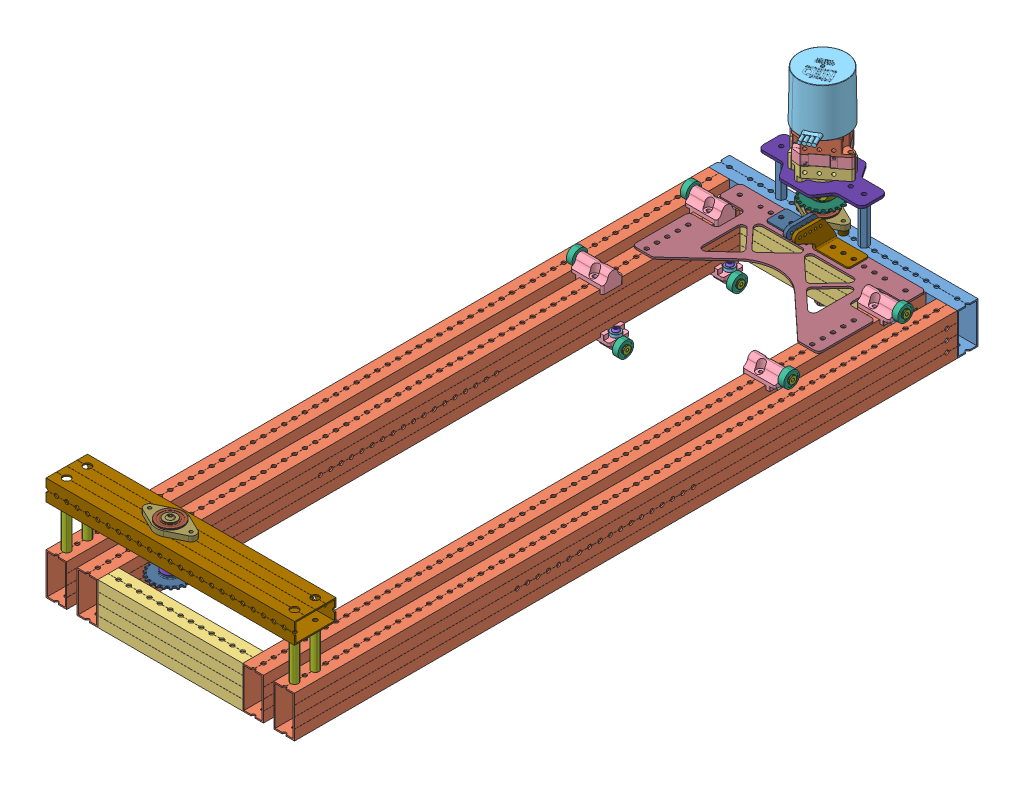
SolidWorks assembly Elevator Assembly Updated 2.0, configuration Default. Lengths in mm.
Overall size (304.8 250.34 871.89).
92 component instances, 31 part files, 131 mates.
Components (placement in the parent):
- WCP-EX-0018-001(2)^Assem1-1: WCP-EX-0018-001(2)^Assem1 [Default] at (184.7308 227.7739 250.3499) size (304.8 50.8 25.4)
- WCP-EX-0018-005(2)^Assem1-1: WCP-EX-0018-005(2)^Assem1 [Default] at (45.0308 227.7739 859.9499) x (0 0 -1) z (1 0 0) size (812.8 50.8 25.4)
- WCP-EX-0018-004(2)^Assem1-1: WCP-EX-0018-004(2)^Assem1 [Default] at (184.7308 227.7739 1063.1499) size (177.8 50.8 25.4)
- WCP-EX-0018-005(2)^Assem1-2: WCP-EX-0018-005(2)^Assem1 [Default] at (324.4308 227.7739 859.9499) x (0 0 -1) z (1 0 0) size (812.8 50.8 25.4)
- WCP-EX-0018-005(2)^Assem1-3: WCP-EX-0018-005(2)^Assem1 [Default] at (286.3308 227.7739 859.9499) x (0 0 -1) z (1 0 0) size (812.8 50.8 25.4)
- WCP-EX-0018-005(2)^Assem1-4: WCP-EX-0018-005(2)^Assem1 [Default] at (83.1308 227.7739 859.9499) x (0 0 -1) z (1 0 0) size (812.8 50.8 25.4)
- WCP-EX-0018-004(2)^Assem1-2: WCP-EX-0018-004(2)^Assem1 [Default] at (184.7308 227.7739 275.7499) size (177.8 50.8 25.4)
- Copy of WCP-0323 - Elevator Clamping Block-1-1: Copy of WCP-0323 - Elevator Clamping Block-1 [Default] at (70.4308 253.1739 307.4999) x (0 -1 0) z (-1 0 0) size (29.22 25.41 49.35)
  - WCP-0323-001 Rev2^Copy of WCP-0323 - Elevator Clamping Block-1-1: WCP-0323-001 Rev2^Copy of WCP-0323 - Elevator Clamping Block-1 [Default] at origin size (20.38 25.41 40.49) (virtual)
  - WCP-0498 Rev1^Copy of WCP-0323 - Elevator Clamping Block-1-1: WCP-0498 Rev1^Copy of WCP-0323 - Elevator Clamping Block-1 [Default] at (2.254 0 6.7) x (0 0.307359 0.951594) z (-1 0 0) size (12 12 4) (virtual)
  - WCP-0212_0_250_radial_bearing^Copy of WCP-0323 - Elevator Clamping Block-1-1: WCP-0212_0_250_radial_bearing^Copy of WCP-0323 - Elevator Clamping Block-1 [Default] at (-9.525 0 15.4781) size (19.05 19.05 7.14) (virtual)
  - WCP-0473 Rev1^Copy of WCP-0323 - Elevator Clamping Block-1-1: WCP-0473 Rev1^Copy of WCP-0323 - Elevator Clamping Block-1 [Default] at (-9.525 0 10.4394) x (-0.082744 -0.996571 0) z (-0.996571 0.082744 0) size (9.53 20.65 9.53) (virtual)
  - #8-32 x .25L BHCS^Copy of WCP-0323 - Elevator Clamping Block-1-1: #8-32 x .25L BHCS^Copy of WCP-0323 - Elevator Clamping Block-1 [Default] at (6.7178 0 6.7) x (0 -0.337236 -0.94142) z (1 0 0) size (10.28 8 12.02) (virtual)
- WCP-0583-025 Rev1_DefaultSM-FLAT-PATTERN(2)^Elevator Assembly Updated 2.0-1: WCP-0583-025 Rev1_DefaultSM-FLAT-PATTERN(2)^Elevator Assembly Updated 2.0 [Default] at (206.9558 257.1739 275.7499) x (-1 0 0) z (0 1 0) size (44.45 50.8 31.75) (virtual)
- WCP-0583-026 Rev1(2)^Elevator Assembly Updated 2.0-1: WCP-0583-026 Rev1(2)^Elevator Assembly Updated 2.0 [Default] at (152.9808 257.1739 275.7499) x (-1 0 0) z (0 1 0) size (50.8 50.8 31.75) (virtual)
- Copy of WCP-0323 - Elevator Clamping Block-1-2: Copy of WCP-0323 - Elevator Clamping Block-1 [Default] at (70.4308 253.1739 447.1999) x (0 -1 0) z (-1 0 0) size (29.22 25.41 49.35)
  - WCP-0323-001 Rev2^Copy of WCP-0323 - Elevator Clamping Block-1-1: WCP-0323-001 Rev2^Copy of WCP-0323 - Elevator Clamping Block-1 [Default] at origin size (20.38 25.41 40.49) (virtual)
  - WCP-0498 Rev1^Copy of WCP-0323 - Elevator Clamping Block-1-1: WCP-0498 Rev1^Copy of WCP-0323 - Elevator Clamping Block-1 [Default] at (2.254 0 6.7) x (0 0.307359 0.951594) z (-1 0 0) size (12 12 4) (virtual)
  - WCP-0212_0_250_radial_bearing^Copy of WCP-0323 - Elevator Clamping Block-1-1: WCP-0212_0_250_radial_bearing^Copy of WCP-0323 - Elevator Clamping Block-1 [Default] at (-9.525 0 15.4781) size (19.05 19.05 7.14) (virtual)
  - WCP-0473 Rev1^Copy of WCP-0323 - Elevator Clamping Block-1-1: WCP-0473 Rev1^Copy of WCP-0323 - Elevator Clamping Block-1 [Default] at (-9.525 0 10.4394) x (-0.082744 -0.996571 0) z (-0.996571 0.082744 0) size (9.53 20.65 9.53) (virtual)
  - #8-32 x .25L BHCS^Copy of WCP-0323 - Elevator Clamping Block-1-1: #8-32 x .25L BHCS^Copy of WCP-0323 - Elevator Clamping Block-1 [Default] at (6.7178 0 6.7) x (0 -0.337236 -0.94142) z (1 0 0) size (10.28 8 12.02) (virtual)
- Copy of WCP-0323 - Elevator Clamping Block-1-3: Copy of WCP-0323 - Elevator Clamping Block-1 [Default] at (299.0308 253.1739 447.1999) x (0 -1 0) z (1 0 0) size (29.22 25.41 49.35)
  - WCP-0323-001 Rev2^Copy of WCP-0323 - Elevator Clamping Block-1-1: WCP-0323-001 Rev2^Copy of WCP-0323 - Elevator Clamping Block-1 [Default] at origin size (20.38 25.41 40.49) (virtual)
  - WCP-0498 Rev1^Copy of WCP-0323 - Elevator Clamping Block-1-1: WCP-0498 Rev1^Copy of WCP-0323 - Elevator Clamping Block-1 [Default] at (2.254 0 6.7) x (0 0.307359 0.951594) z (-1 0 0) size (12 12 4) (virtual)
  - WCP-0212_0_250_radial_bearing^Copy of WCP-0323 - Elevator Clamping Block-1-1: WCP-0212_0_250_radial_bearing^Copy of WCP-0323 - Elevator Clamping Block-1 [Default] at (-9.525 0 15.4781) size (19.05 19.05 7.14) (virtual)
  - WCP-0473 Rev1^Copy of WCP-0323 - Elevator Clamping Block-1-1: WCP-0473 Rev1^Copy of WCP-0323 - Elevator Clamping Block-1 [Default] at (-9.525 0 10.4394) x (-0.082744 -0.996571 0) z (-0.996571 0.082744 0) size (9.53 20.65 9.53) (virtual)
  - #8-32 x .25L BHCS^Copy of WCP-0323 - Elevator Clamping Block-1-1: #8-32 x .25L BHCS^Copy of WCP-0323 - Elevator Clamping Block-1 [Default] at (6.7178 0 6.7) x (0 -0.337236 -0.94142) z (1 0 0) size (10.28 8 12.02) (virtual)
- Copy of WCP-0323 - Elevator Clamping Block-1-4: Copy of WCP-0323 - Elevator Clamping Block-1 [Default] at (299.0308 253.1739 307.4999) x (0 -1 0) z (1 0 0) size (29.22 25.41 49.35)
  - WCP-0323-001 Rev2^Copy of WCP-0323 - Elevator Clamping Block-1-1: WCP-0323-001 Rev2^Copy of WCP-0323 - Elevator Clamping Block-1 [Default] at origin size (20.38 25.41 40.49) (virtual)
  - WCP-0498 Rev1^Copy of WCP-0323 - Elevator Clamping Block-1-1: WCP-0498 Rev1^Copy of WCP-0323 - Elevator Clamping Block-1 [Default] at (2.254 0 6.7) x (0 0.307359 0.951594) z (-1 0 0) size (12 12 4) (virtual)
  - WCP-0212_0_250_radial_bearing^Copy of WCP-0323 - Elevator Clamping Block-1-1: WCP-0212_0_250_radial_bearing^Copy of WCP-0323 - Elevator Clamping Block-1 [Default] at (-9.525 0 15.4781) size (19.05 19.05 7.14) (virtual)
  - WCP-0473 Rev1^Copy of WCP-0323 - Elevator Clamping Block-1-1: WCP-0473 Rev1^Copy of WCP-0323 - Elevator Clamping Block-1 [Default] at (-9.525 0 10.4394) x (-0.082744 -0.996571 0) z (-0.996571 0.082744 0) size (9.53 20.65 9.53) (virtual)
  - #8-32 x .25L BHCS^Copy of WCP-0323 - Elevator Clamping Block-1-1: #8-32 x .25L BHCS^Copy of WCP-0323 - Elevator Clamping Block-1 [Default] at (6.7178 0 6.7) x (0 -0.337236 -0.94142) z (1 0 0) size (10.28 8 12.02) (virtual)
- Copy of WCP-0323 - Elevator Clamping Block-1-5: Copy of WCP-0323 - Elevator Clamping Block-1 [Default] at (95.9578 202.3739 307.4999) x (0 1 0) z (1 0 0) size (29.22 25.41 49.35)
  - WCP-0323-001 Rev2^Copy of WCP-0323 - Elevator Clamping Block-1-1: WCP-0323-001 Rev2^Copy of WCP-0323 - Elevator Clamping Block-1 [Default] at origin size (20.38 25.41 40.49) (virtual)
  - WCP-0498 Rev1^Copy of WCP-0323 - Elevator Clamping Block-1-1: WCP-0498 Rev1^Copy of WCP-0323 - Elevator Clamping Block-1 [Default] at (2.254 0 6.7) x (0 0.307359 0.951594) z (-1 0 0) size (12 12 4) (virtual)
  - WCP-0212_0_250_radial_bearing^Copy of WCP-0323 - Elevator Clamping Block-1-1: WCP-0212_0_250_radial_bearing^Copy of WCP-0323 - Elevator Clamping Block-1 [Default] at (-9.525 0 15.4781) size (19.05 19.05 7.14) (virtual)
  - WCP-0473 Rev1^Copy of WCP-0323 - Elevator Clamping Block-1-1: WCP-0473 Rev1^Copy of WCP-0323 - Elevator Clamping Block-1 [Default] at (-9.525 0 10.4394) x (-0.082744 -0.996571 0) z (-0.996571 0.082744 0) size (9.53 20.65 9.53) (virtual)
  - #8-32 x .25L BHCS^Copy of WCP-0323 - Elevator Clamping Block-1-1: #8-32 x .25L BHCS^Copy of WCP-0323 - Elevator Clamping Block-1 [Default] at (6.7178 0 6.7) x (0 -0.337236 -0.94142) z (1 0 0) size (10.28 8 12.02) (virtual)
- Copy of WCP-0323 - Elevator Clamping Block-1-6: Copy of WCP-0323 - Elevator Clamping Block-1 [Default] at (299.1578 202.3739 447.1999) x (0 1 0) z (1 0 0) size (29.22 25.41 49.35)
  - WCP-0323-001 Rev2^Copy of WCP-0323 - Elevator Clamping Block-1-1: WCP-0323-001 Rev2^Copy of WCP-0323 - Elevator Clamping Block-1 [Default] at origin size (20.38 25.41 40.49) (virtual)
  - WCP-0498 Rev1^Copy of WCP-0323 - Elevator Clamping Block-1-1: WCP-0498 Rev1^Copy of WCP-0323 - Elevator Clamping Block-1 [Default] at (2.254 0 6.7) x (0 0.307359 0.951594) z (-1 0 0) size (12 12 4) (virtual)
  - WCP-0212_0_250_radial_bearing^Copy of WCP-0323 - Elevator Clamping Block-1-1: WCP-0212_0_250_radial_bearing^Copy of WCP-0323 - Elevator Clamping Block-1 [Default] at (-9.525 0 15.4781) size (19.05 19.05 7.14) (virtual)
  - WCP-0473 Rev1^Copy of WCP-0323 - Elevator Clamping Block-1-1: WCP-0473 Rev1^Copy of WCP-0323 - Elevator Clamping Block-1 [Default] at (-9.525 0 10.4394) x (-0.082744 -0.996571 0) z (-0.996571 0.082744 0) size (9.53 20.65 9.53) (virtual)
  - #8-32 x .25L BHCS^Copy of WCP-0323 - Elevator Clamping Block-1-1: #8-32 x .25L BHCS^Copy of WCP-0323 - Elevator Clamping Block-1 [Default] at (6.7178 0 6.7) x (0 -0.337236 -0.94142) z (1 0 0) size (10.28 8 12.02) (virtual)
- Copy of WCP-0323 - Elevator Clamping Block-1-7: Copy of WCP-0323 - Elevator Clamping Block-1 [Default] at (299.1578 202.3739 307.4999) x (0 1 0) z (1 0 0) size (29.22 25.41 49.35)
  - WCP-0323-001 Rev2^Copy of WCP-0323 - Elevator Clamping Block-1-1: WCP-0323-001 Rev2^Copy of WCP-0323 - Elevator Clamping Block-1 [Default] at origin size (20.38 25.41 40.49) (virtual)
  - WCP-0498 Rev1^Copy of WCP-0323 - Elevator Clamping Block-1-1: WCP-0498 Rev1^Copy of WCP-0323 - Elevator Clamping Block-1 [Default] at (2.254 0 6.7) x (0 0.307359 0.951594) z (-1 0 0) size (12 12 4) (virtual)
  - WCP-0212_0_250_radial_bearing^Copy of WCP-0323 - Elevator Clamping Block-1-1: WCP-0212_0_250_radial_bearing^Copy of WCP-0323 - Elevator Clamping Block-1 [Default] at (-9.525 0 15.4781) size (19.05 19.05 7.14) (virtual)
  - WCP-0473 Rev1^Copy of WCP-0323 - Elevator Clamping Block-1-1: WCP-0473 Rev1^Copy of WCP-0323 - Elevator Clamping Block-1 [Default] at (-9.525 0 10.4394) x (-0.082744 -0.996571 0) z (-0.996571 0.082744 0) size (9.53 20.65 9.53) (virtual)
  - #8-32 x .25L BHCS^Copy of WCP-0323 - Elevator Clamping Block-1-1: #8-32 x .25L BHCS^Copy of WCP-0323 - Elevator Clamping Block-1 [Default] at (6.7178 0 6.7) x (0 -0.337236 -0.94142) z (1 0 0) size (10.28 8 12.02) (virtual)
- Copy of WCP-0323 - Elevator Clamping Block-1-8: Copy of WCP-0323 - Elevator Clamping Block-1 [Default] at (95.8308 202.3739 447.1999) x (0 1 0) z (1 0 0) size (29.22 25.41 49.35)
  - WCP-0323-001 Rev2^Copy of WCP-0323 - Elevator Clamping Block-1-1: WCP-0323-001 Rev2^Copy of WCP-0323 - Elevator Clamping Block-1 [Default] at origin size (20.38 25.41 40.49) (virtual)
  - WCP-0498 Rev1^Copy of WCP-0323 - Elevator Clamping Block-1-1: WCP-0498 Rev1^Copy of WCP-0323 - Elevator Clamping Block-1 [Default] at (2.254 0 6.7) x (0 0.307359 0.951594) z (-1 0 0) size (12 12 4) (virtual)
  - WCP-0212_0_250_radial_bearing^Copy of WCP-0323 - Elevator Clamping Block-1-1: WCP-0212_0_250_radial_bearing^Copy of WCP-0323 - Elevator Clamping Block-1 [Default] at (-9.525 0 15.4781) size (19.05 19.05 7.14) (virtual)
  - WCP-0473 Rev1^Copy of WCP-0323 - Elevator Clamping Block-1-1: WCP-0473 Rev1^Copy of WCP-0323 - Elevator Clamping Block-1 [Default] at (-9.525 0 10.4394) x (-0.082744 -0.996571 0) z (-0.996571 0.082744 0) size (9.53 20.65 9.53) (virtual)
  - #8-32 x .25L BHCS^Copy of WCP-0323 - Elevator Clamping Block-1-1: #8-32 x .25L BHCS^Copy of WCP-0323 - Elevator Clamping Block-1 [Default] at (6.7178 0 6.7) x (0 -0.337236 -0.94142) z (1 0 0) size (10.28 8 12.02) (virtual)
- WCP-0785_0_500_flanged_thunderhex_bearing.step-1: WCP-0785_0_500_flanged_thunderhex_bearing.step [Default] at (159.3308 263.4926 250.3499) x (0.189996 0 -0.981785) z (0 1 0) size (31.12 31.12 7.94)
- Copy of WCP-0476 Rev1^Elevator Assembly Updated 2.0-1: Copy of WCP-0476 Rev1^Elevator Assembly Updated 2.0 [Default] at (159.3308 262.6989 250.3499) x (1 0 0) z (0 -1 0) size (63.5 34.92 6.35) (virtual)
- 1_2ThunderHex-1: 1_2ThunderHex [Default] at (159.3308 624.6489 250.3499) x (0.958899 0 0.283749) z (0 1 0) size (13.74 12.75 152.4)
- Copy of WCP-0789_250L_500_hex^Elevator Assembly Updated 2.0-1: Copy of WCP-0789_250L_500_hex^Elevator Assembly Updated 2.0 [Default] at (159.3308 270.6364 250.3499) x (0.725183 0 -0.688556) z (0 1 0) size (19.5 19.5 6.35) (virtual)
- Copy of WCP-0560 Rev1^Elevator Assembly Updated 2.0-1: Copy of WCP-0560 Rev1^Elevator Assembly Updated 2.0 [Default] at (159.3308 278.5739 250.3499) x (-0.972305 0 0.233715) z (0 -1 0) size (47.96 47.68 9.53) (virtual)
- Copy of WCP-0800_500_hex_collar_high_strength^Elevator Assembly Updated 2.0-1: Copy of WCP-0800_500_hex_collar_high_strength^Elevator Assembly Updated 2.0 [Default] at (159.3308 288.0989 250.3499) x (-0.013608 0 0.999907) z (0 1 0) size (28.56 28.57 9.53) (virtual)
- Motor_Mounting_Plate-1: Motor_Mounting_Plate [Default] at (108.5308 307.1489 250.3499) x (1 0 0) z (0 0 -1) size (127 3.17 69.85)
- Copy of WCP-0308 Rev1^Elevator Assembly Updated 2.0-1: Copy of WCP-0308 Rev1^Elevator Assembly Updated 2.0 [Default] at (184.7308 256.3489 250.3499) x (0 1 0) z (0.995626 0 0.093431) size (6.35 9.5 9.5) (virtual)
- 2in_Standoff-1: 2in_Standoff [Default] at (108.5308 278.5739 250.3499) x (0 -1 0) z (0.316201 0 -0.948692) size (50.8 9.53 11)
- Copy of WCP-0308 Rev1^Elevator Assembly Updated 2.0-2: Copy of WCP-0308 Rev1^Elevator Assembly Updated 2.0 [Default] at (133.9308 256.3489 250.3499) x (0 1 0) z (0.99 0 0.141064) size (6.35 9.5 9.5) (virtual)
- 2in_Standoff-2: 2in_Standoff [Default] at (210.1308 278.5739 250.3499) x (0 -1 0) z (-0.228411 0 -0.973565) size (50.8 9.53 11)
- WCP-0785_0_500_flanged_thunderhex_bearing.step-2: WCP-0785_0_500_flanged_thunderhex_bearing.step [Default] at (159.3308 304.7676 250.3499) x (0.067794 0 0.997699) z (0 1 0) size (31.12 31.12 7.94)
- REV-21-2106-universal-input-1: REV-21-2106-universal-input [Default] at (159.3273 349.9114 250.3526) x (0.784058 0 -0.620687) z (0 -1 0) size (61.91 50.8 19.05)
- REV-21-2104-hex-socket-output-1: REV-21-2104-hex-socket-output [Default] at (159.3308 318.2614 250.3499) x (0 -1 0) z (-0.784058 0 0.620687) size (23.2 50.8 61.92)
- REV-21-2102-4-1-cartridge-1: REV-21-2102-4-1-cartridge [Default] at (159.3273 334.0864 250.3526) x (0.784058 0 -0.620687) z (0 -1 0) size (61.91 50.8 16.85)
- Neo1.1_REV-21-1650-V1.1-1: Neo1.1_REV-21-1650-V1.1 [Default] at (159.3273 359.4364 250.3526) x (0.308177 0 -0.951329) z (0 -1 0) size (68.13 68.01 93.35)
- WCP-0785_0_500_flanged_thunderhex_bearing.step-3: WCP-0785_0_500_flanged_thunderhex_bearing.step [Default] at (159.3308 192.0551 250.3499) x (-0.762178 0 -0.647368) z (0 -1 0) size (31.12 31.12 7.94)
- Copy (2) of WCP-0476 Rev1^Elevator Assembly Updated 2.0-1: Copy (2) of WCP-0476 Rev1^Elevator Assembly Updated 2.0 [Default] at (159.3308 192.8489 250.3499) x (0.999931 0 0.011762) z (0 1 0) size (63.5 34.92 6.35) (virtual)
- Copy of WCP-0308 Rev1^Elevator Assembly Updated 2.0-4: Copy of WCP-0308 Rev1^Elevator Assembly Updated 2.0 [Default] at (184.729 199.1989 250.6486) x (0 1 0) z (0.995626 0 0.093431) size (6.35 9.5 9.5) (virtual)
- Copy of WCP-0308 Rev1^Elevator Assembly Updated 2.0-5: Copy of WCP-0308 Rev1^Elevator Assembly Updated 2.0 [Default] at (133.9325 199.1989 250.0511) x (0 1 0) z (0.995626 0 0.093431) size (6.35 9.5 9.5) (virtual)
- Copy of WCP-0207 Rev1^Elevator Assembly Updated 2.0-1: Copy of WCP-0207 Rev1^Elevator Assembly Updated 2.0 [Default] at (45.0308 278.5739 1063.1499) x (0 -1 0) z (0.710119 0 0.704082) size (50.8 9.5 9.5) (virtual)
- WCP-0790_500L_500_hex.step-1: WCP-0790_500L_500_hex.step [Default] at (159.3308 289.6864 1050.4499) x (0.992611 0 -0.121342) z (0 -1 0) size (19.5 19.5 12.7)
- WCP-EX-0018-002(2)^Elevator Assembly Updated 2.0-1: WCP-EX-0018-002(2)^Elevator Assembly Updated 2.0 [Default] at (184.7308 316.6739 1050.4499) x (1 0 0) z (0 -1 0) size (304.8 50.8 25.4)
- Copy of WCP-0207 Rev1^Elevator Assembly Updated 2.0-2: Copy of WCP-0207 Rev1^Elevator Assembly Updated 2.0 [Default] at (324.4308 278.5739 1037.7499) x (0 -1 0) z (0.909972 0 0.414669) size (50.8 9.5 9.5) (virtual)
- Copy of WCP-0207 Rev1^Elevator Assembly Updated 2.0-3: Copy of WCP-0207 Rev1^Elevator Assembly Updated 2.0 [Default] at (45.0308 278.5739 1037.7499) x (0 -1 0) z (-0.997465 0 0.071155) size (50.8 9.5 9.5) (virtual)
- Copy of WCP-0207 Rev1^Elevator Assembly Updated 2.0-4: Copy of WCP-0207 Rev1^Elevator Assembly Updated 2.0 [Default] at (324.4308 278.5739 1063.1499) x (0 -1 0) z (-0.448341 0 -0.893863) size (50.8 9.5 9.5) (virtual)
- Copy of WCP-0476 Rev1^Elevator Assembly Updated 2.0-2: Copy of WCP-0476 Rev1^Elevator Assembly Updated 2.0 [Default] at (159.3308 332.5489 1050.4499) x (1 0 0) z (0 -1 0) size (63.5 34.92 6.35) (virtual)
- WCP-0785_0_500_flanged_thunderhex_bearing.step-4: WCP-0785_0_500_flanged_thunderhex_bearing.step [Default] at (159.3308 333.3426 1050.4499) x (0.679938 0 -0.73327) z (0 1 0) size (31.12 31.12 7.94)
- Copy of WCP-0476 Rev1^Elevator Assembly Updated 2.0-4: Copy of WCP-0476 Rev1^Elevator Assembly Updated 2.0 [Default] at (159.3308 300.7989 1050.4499) x (1 0 0) z (0 1 0) size (63.5 34.92 6.35) (virtual)
- WCP-0785_0_500_flanged_thunderhex_bearing.step-6: WCP-0785_0_500_flanged_thunderhex_bearing.step [Default] at (159.3308 300.0051 1050.4499) x (-0.189996 0 -0.981785) z (0 -1 0) size (31.12 31.12 7.94)
- Copy (2) of WCP-0560 Rev1^Elevator Assembly Updated 2.0-2: Copy (2) of WCP-0560 Rev1^Elevator Assembly Updated 2.0 [Default] at (159.3308 278.5739 1050.4499) x (-0.499725 0 -0.866184) z (0 -1 0) size (47.96 47.68 9.53) (virtual)
- Copy of WCP-0599 Rev1^Elevator Assembly Updated 2.0-1: Copy of WCP-0599 Rev1^Elevator Assembly Updated 2.0 [Default] at (159.3308 305.5614 1050.4499) x (0 -1 0) z (-0.000318 0 1) size (63.5 12.67 13.72) (virtual)
- Copy of WCP-0571 Rev1^Elevator Assembly Updated 2.0-1: Copy of WCP-0571 Rev1^Elevator Assembly Updated 2.0 [Default] at (159.3308 270.8142 1050.4499) x (-0.946289 0 0.323321) z (0 -1 0) size (15.88 15.88 15.71) (virtual)
- Copy of WCP-0571 Rev1^Elevator Assembly Updated 2.0-2: Copy of WCP-0571 Rev1^Elevator Assembly Updated 2.0 [Default] at (159.3308 340.3086 1050.4499) x (-0.49457 0 -0.869138) z (0 1 0) size (15.88 15.88 15.71) (virtual)
- Part3^Elevator Assembly Updated 2.0-1: Part3^Elevator Assembly Updated 2.0 [Default] at (83.1308 253.1739 859.9499) x (0 0 -1) z (0 1 0) size (132.08 228.6 2.29) (virtual)
Mates (geometry in assembly coordinates):
- Coincident1: coincident: plane of WCP-EX-0018-005(2)^Assem1-1 through (45.0308 227.7739 263.0499) normal (0 0 -1); line of WCP-EX-0018-005(2)^Assem1-2 through (313.3183 251.5864 263.0499) axis (1 0 0)
- Coincident2: coincident aligned: plane of WCP-EX-0018-005(2)^Assem1-1 through (57.7308 253.1739 263.0499) normal (0 1 0); plane of WCP-EX-0018-005(2)^Assem1-2 through (337.1308 253.1739 263.0499) normal (0 1 0)
- Distance1: distance = 304.8 mm anti-aligned: plane of WCP-EX-0018-005(2)^Assem1-2 through (337.1308 202.3739 263.0499) normal (1 0 0); plane of WCP-EX-0018-005(2)^Assem1-1 through (32.3308 202.3739 263.0499) normal (-1 0 0)
- Coincident4: coincident anti-aligned: plane of WCP-EX-0018-001(2)^Assem1-1 through (375.2308 202.3739 263.0499) normal (0 0 1); plane of WCP-EX-0018-005(2)^Assem1-1 through (45.0308 227.7739 263.0499) normal (0 0 -1)
- Coincident5: coincident: line of WCP-EX-0018-001(2)^Assem1-1 through (337.1308 253.1739 263.0499) axis (-1 0 0); plane of WCP-EX-0018-005(2)^Assem1-1 through (57.7308 253.1739 263.0499) normal (0 1 0)
- Coincident7: coincident aligned: plane of WCP-EX-0018-005(2)^Assem1-3 through (299.0308 253.1739 263.0499) normal (0 1 0); plane of WCP-EX-0018-005(2)^Assem1-4 through (95.8308 253.1739 263.0499) normal (0 1 0)
- Coincident8: coincident: line of WCP-EX-0018-005(2)^Assem1-3 through (275.2183 251.5864 263.0499) axis (1 0 0); plane of WCP-EX-0018-005(2)^Assem1-4 through (83.1308 227.7739 263.0499) normal (0 0 -1)
- Distance3: distance = 228.6 mm anti-aligned: plane of WCP-EX-0018-005(2)^Assem1-3 through (299.0308 202.3739 263.0499) normal (1 0 0); plane of WCP-EX-0018-005(2)^Assem1-4 through (70.4308 202.3739 263.0499) normal (-1 0 0)
- Coincident9: coincident aligned: plane of WCP-EX-0018-001(2)^Assem1-1 through (375.2308 253.1739 263.0499) normal (0 1 0); plane of WCP-EX-0018-005(2)^Assem1-4 through (95.8308 253.1739 263.0499) normal (0 1 0)
- Distance4: distance = 12.7 mm anti-aligned: plane of WCP-EX-0018-005(2)^Assem1-1 through (57.7308 202.3739 263.0499) normal (1 0 0); plane of WCP-EX-0018-005(2)^Assem1-4 through (70.4308 202.3739 263.0499) normal (-1 0 0)
- Coincident12: coincident: plane of WCP-EX-0018-001(2)^Assem1-1 through (375.2308 202.3739 263.0499) normal (0 0 1); line of WCP-EX-0018-005(2)^Assem1-4 through (83.207 253.1739 263.0499) axis (1 0 0)
- Coincident13: coincident aligned: plane of WCP-EX-0018-005(2)^Assem1-1 through (57.7308 253.1739 263.0499) normal (0 1 0); plane of WCP-EX-0018-004(2)^Assem1-1 through (260.9308 253.1739 1075.8499) normal (0 1 0)
- Coincident14: coincident: line of WCP-EX-0018-004(2)^Assem1-1 through (273.6308 253.1739 1063.2261) axis (0 0 1); plane of WCP-EX-0018-005(2)^Assem1-3 through (273.6308 202.3739 263.0499) normal (-1 0 0)
- Coincident18: coincident: plane of WCP-EX-0018-001(2)^Assem1-1 through (375.2308 253.1739 263.0499) normal (0 1 0); line of WCP-EX-0018-004(2)^Assem1-2 through (273.6308 253.1739 263.0499) axis (-1 0 0)
- Coincident19: coincident anti-aligned: plane of WCP-EX-0018-001(2)^Assem1-1 through (375.2308 202.3739 263.0499) normal (0 0 1); plane of WCP-EX-0018-004(2)^Assem1-2 through (260.9308 202.3739 263.0499) normal (0 0 -1)
- Coincident20: coincident anti-aligned: plane of WCP-EX-0018-005(2)^Assem1-3 through (273.6308 202.3739 263.0499) normal (-1 0 0); plane of WCP-EX-0018-004(2)^Assem1-2 through (273.6308 227.7739 275.7499) normal (1 0 0)
- Coincident21: coincident anti-aligned: plane of WCP-EX-0018-004(2)^Assem1-2 through (260.9308 253.1739 288.4499) normal (0 1 0); plane of WCP-0583-025 Rev1_DefaultSM-FLAT-PATTERN.step-1 through (206.9558 253.1739 275.7499) normal (0 -1 0)
- Coincident22: coincident anti-aligned: plane of WCP-EX-0018-004(2)^Assem1-2 through (260.9308 253.1739 288.4499) normal (0 1 0); plane of WCP-0583-026 Rev1.step-1 through (152.9808 253.1739 275.7499) normal (0 -1 0)
- Concentric1: concentric aligned: circle of WCP-EX-0018-004(2)^Assem1-2; cylinder of WCP-0583-026 Rev1.step-1 through (159.3308 253.1739 275.7499) axis (0 1 0) radius 2.4892
- Concentric2: concentric aligned: cylinder of WCP-EX-0018-004(2)^Assem1-2 through (197.4308 202.3739 275.7499) axis (0 1 0) radius 2.4892; cylinder of WCP-0583-025 Rev1_DefaultSM-FLAT-PATTERN.step-1 through (197.4308 253.1739 275.7499) axis (0 1 0) radius 2.4892
- Parallel2: parallel anti-aligned: plane of WCP-0583-025 Rev1_DefaultSM-FLAT-PATTERN.step-1 through (184.7308 258.7614 269.3999) normal (-1 0 0); plane of WCP-0583-026 Rev1.step-1 through (178.3808 258.7614 294.7999) normal (1 0 0)
- Coincident24: coincident: plane of WCP-EX-0018-004(2)^Assem1-2 through (260.9308 202.3739 288.4499) normal (0 0 1); line of WCP-0583-026 Rev1.step-1 through (130.7558 257.1739 288.4499) axis (1 0 0)
- Coincident25: coincident anti-aligned: plane of WCP-EX-0018-005(2)^Assem1-4 through (95.8308 253.1739 263.0499) normal (0 1 0); plane of Copy of WCP-0323 - Elevator Clamping Block-1-1/WCP-0323-001 Rev2^Copy of WCP-0323 - Elevator Clamping Block-1-1 through (70.4308 253.1739 307.4999) normal (0 -1 0)
- Coincident26: coincident anti-aligned: plane of WCP-EX-0018-005(2)^Assem1-4 through (70.4308 202.3739 263.0499) normal (-1 0 0); plane of Copy of WCP-0323 - Elevator Clamping Block-1-1/WCP-0323-001 Rev2^Copy of WCP-0323 - Elevator Clamping Block-1-1 through (70.4308 248.6659 307.4999) normal (1 0 0)
- Coincident28: coincident anti-aligned: plane of WCP-EX-0018-005(2)^Assem1-4 through (70.4308 202.3739 263.0499) normal (-1 0 0); plane of Copy of WCP-0323 - Elevator Clamping Block-1-2/WCP-0323-001 Rev2^Copy of WCP-0323 - Elevator Clamping Block-1-1 through (70.4308 248.6659 447.1999) normal (1 0 0)
- Coincident29: coincident: plane of WCP-EX-0018-005(2)^Assem1-4 through (95.8308 253.1739 263.0499) normal (0 1 0); line of Copy of WCP-0323 - Elevator Clamping Block-1-2/WCP-0323-001 Rev2^Copy of WCP-0323 - Elevator Clamping Block-1-1 through (95.9578 253.1739 459.8999) axis (-1 0 0)
- Coincident30: coincident anti-aligned: plane of WCP-EX-0018-005(2)^Assem1-3 through (299.0308 202.3739 263.0499) normal (1 0 0); plane of Copy of WCP-0323 - Elevator Clamping Block-1-4/WCP-0323-001 Rev2^Copy of WCP-0323 - Elevator Clamping Block-1-1 through (299.0308 248.6659 307.4999) normal (-1 0 0)
- Coincident31: coincident anti-aligned: plane of WCP-EX-0018-005(2)^Assem1-3 through (299.0308 253.1739 263.0499) normal (0 1 0); plane of Copy of WCP-0323 - Elevator Clamping Block-1-4/WCP-0323-001 Rev2^Copy of WCP-0323 - Elevator Clamping Block-1-1 through (299.0308 253.1739 307.4999) normal (0 -1 0)
- Coincident32: coincident anti-aligned: plane of WCP-EX-0018-005(2)^Assem1-3 through (299.0308 202.3739 263.0499) normal (1 0 0); plane of Copy of WCP-0323 - Elevator Clamping Block-1-3/WCP-0323-001 Rev2^Copy of WCP-0323 - Elevator Clamping Block-1-1 through (299.0308 248.6659 447.1999) normal (-1 0 0)
- Coincident33: coincident anti-aligned: plane of WCP-EX-0018-005(2)^Assem1-3 through (299.0308 253.1739 263.0499) normal (0 1 0); plane of Copy of WCP-0323 - Elevator Clamping Block-1-3/WCP-0323-001 Rev2^Copy of WCP-0323 - Elevator Clamping Block-1-1 through (299.0308 253.1739 447.1999) normal (0 -1 0)
- Coincident36: coincident anti-aligned: plane of WCP-EX-0018-005(2)^Assem1-3 through (299.0308 202.3739 263.0499) normal (0 -1 0); plane of Copy of WCP-0323 - Elevator Clamping Block-1-6/WCP-0323-001 Rev2^Copy of WCP-0323 - Elevator Clamping Block-1-1 through (299.1578 202.3739 447.1999) normal (0 1 0)
- Coincident37: coincident anti-aligned: plane of WCP-EX-0018-005(2)^Assem1-3 through (273.6308 202.3739 263.0499) normal (-1 0 0); plane of Copy of WCP-0323 - Elevator Clamping Block-1-6/WCP-0323-001 Rev2^Copy of WCP-0323 - Elevator Clamping Block-1-1 through (273.6308 206.8819 447.1999) normal (1 0 0)
- Coincident38: coincident anti-aligned: plane of WCP-EX-0018-005(2)^Assem1-3 through (299.0308 202.3739 263.0499) normal (0 -1 0); plane of Copy of WCP-0323 - Elevator Clamping Block-1-7/WCP-0323-001 Rev2^Copy of WCP-0323 - Elevator Clamping Block-1-1 through (299.1578 202.3739 307.4999) normal (0 1 0)
- Coincident39: coincident anti-aligned: plane of WCP-EX-0018-005(2)^Assem1-3 through (273.6308 202.3739 263.0499) normal (-1 0 0); plane of Copy of WCP-0323 - Elevator Clamping Block-1-7/WCP-0323-001 Rev2^Copy of WCP-0323 - Elevator Clamping Block-1-1 through (273.6308 206.8819 307.4999) normal (1 0 0)
- Coincident40: coincident anti-aligned: plane of WCP-EX-0018-005(2)^Assem1-4 through (95.8308 202.3739 263.0499) normal (0 -1 0); plane of Copy of WCP-0323 - Elevator Clamping Block-1-5/WCP-0323-001 Rev2^Copy of WCP-0323 - Elevator Clamping Block-1-1 through (95.9578 202.3739 307.4999) normal (0 1 0)
- Coincident41: coincident anti-aligned: plane of WCP-EX-0018-005(2)^Assem1-4 through (70.4308 202.3739 263.0499) normal (-1 0 0); plane of Copy of WCP-0323 - Elevator Clamping Block-1-5/WCP-0323-001 Rev2^Copy of WCP-0323 - Elevator Clamping Block-1-1 through (70.4308 206.8819 307.4999) normal (1 0 0)
- Coincident42: coincident anti-aligned: plane of WCP-EX-0018-005(2)^Assem1-4 through (95.8308 202.3739 263.0499) normal (1 0 0); plane of Copy of WCP-0323 - Elevator Clamping Block-1-8/WCP-0323-001 Rev2^Copy of WCP-0323 - Elevator Clamping Block-1-1 through (95.8308 206.8819 447.1999) normal (-1 0 0)
- Coincident43: coincident anti-aligned: plane of WCP-EX-0018-005(2)^Assem1-1 through (57.7308 202.3739 263.0499) normal (0 -1 0); plane of Copy of WCP-0323 - Elevator Clamping Block-1-8/WCP-0323-001 Rev2^Copy of WCP-0323 - Elevator Clamping Block-1-1 through (95.8308 202.3739 447.1999) normal (0 1 0)
- Coincident45: coincident aligned: plane of Copy of WCP-0323 - Elevator Clamping Block-1-4/WCP-0323-001 Rev2^Copy of WCP-0323 - Elevator Clamping Block-1-1 through (310.937 253.1739 294.7999) normal (0 0 -1); plane of Copy of WCP-0323 - Elevator Clamping Block-1-7/WCP-0323-001 Rev2^Copy of WCP-0323 - Elevator Clamping Block-1-1 through (311.064 202.3739 294.7999) normal (0 0 -1)
- Coincident46: coincident aligned: plane of Copy of WCP-0323 - Elevator Clamping Block-1-3/WCP-0323-001 Rev2^Copy of WCP-0323 - Elevator Clamping Block-1-1 through (310.937 253.1739 434.4999) normal (0 0 -1); plane of Copy of WCP-0323 - Elevator Clamping Block-1-6/WCP-0323-001 Rev2^Copy of WCP-0323 - Elevator Clamping Block-1-1 through (311.064 202.3739 434.4999) normal (0 0 -1)
- Coincident47: coincident aligned: plane of Copy of WCP-0323 - Elevator Clamping Block-1-1/WCP-0323-001 Rev2^Copy of WCP-0323 - Elevator Clamping Block-1-1 through (58.5245 253.1739 294.7999) normal (0 0 -1); plane of Copy of WCP-0323 - Elevator Clamping Block-1-4/WCP-0323-001 Rev2^Copy of WCP-0323 - Elevator Clamping Block-1-1 through (310.937 253.1739 294.7999) normal (0 0 -1)
- Coincident48: coincident aligned: plane of Copy of WCP-0323 - Elevator Clamping Block-1-2/WCP-0323-001 Rev2^Copy of WCP-0323 - Elevator Clamping Block-1-1 through (58.5245 253.1739 434.4999) normal (0 0 -1); plane of Copy of WCP-0323 - Elevator Clamping Block-1-3/WCP-0323-001 Rev2^Copy of WCP-0323 - Elevator Clamping Block-1-1 through (310.937 253.1739 434.4999) normal (0 0 -1)
- Coincident49: coincident aligned: plane of Copy of WCP-0323 - Elevator Clamping Block-1-1/WCP-0323-001 Rev2^Copy of WCP-0323 - Elevator Clamping Block-1-1 through (58.5245 253.1739 294.7999) normal (0 0 -1); plane of Copy of WCP-0323 - Elevator Clamping Block-1-5/WCP-0323-001 Rev2^Copy of WCP-0323 - Elevator Clamping Block-1-1 through (107.864 202.3739 294.7999) normal (0 0 -1)
- Coincident51: coincident aligned: plane of Copy of WCP-0323 - Elevator Clamping Block-1-2/WCP-0323-001 Rev2^Copy of WCP-0323 - Elevator Clamping Block-1-1 through (58.5245 253.1739 434.4999) normal (0 0 -1); plane of Copy of WCP-0323 - Elevator Clamping Block-1-8/WCP-0323-001 Rev2^Copy of WCP-0323 - Elevator Clamping Block-1-1 through (107.737 202.3739 434.4999) normal (0 0 -1)
- Concentric6: concentric anti-aligned: cylinder of WCP-EX-0018-001(2)^Assem1-1 through (184.7308 202.3739 250.3499) axis (0 1 0) radius 2.4892; cylinder of Copy of WCP-0476 Rev1^Elevator Assembly Updated 2.0-1 through (184.7308 259.5239 250.3499) axis (0 -1 0) radius 2.0193
- Concentric7: concentric anti-aligned: cylinder of WCP-EX-0018-001(2)^Assem1-1 through (133.9308 202.3739 250.3499) axis (0 1 0) radius 2.4892; circle of Copy of WCP-0476 Rev1^Elevator Assembly Updated 2.0-1
- Concentric8: concentric aligned: cylinder of WCP-0785_0_500_flanged_thunderhex_bearing.step-1 through (159.3308 316.7416 250.3499) axis (0 1 0) radius 14.2875; cylinder of Copy of WCP-0476 Rev1^Elevator Assembly Updated 2.0-1 through (159.3308 259.5239 250.3499) axis (0 1 0) radius 14.2875
- Coincident54: coincident anti-aligned: plane of WCP-0785_0_500_flanged_thunderhex_bearing.step-1 through (145.3035 265.8739 247.6353) normal (0 -1 0); plane of Copy of WCP-0476 Rev1^Elevator Assembly Updated 2.0-1 through (159.3308 265.8739 250.3499) normal (0 1 0)
- Concentric9: concentric aligned: cylinder of 1_2ThunderHex-1 through (159.3308 167.4489 250.3499) axis (0 1 0) radius 2.55; circle of Copy of WCP-0800_500_hex_collar_high_strength^Elevator Assembly Updated 2.0-1
- Concentric10: concentric anti-aligned: cylinder of WCP-0785_0_500_flanged_thunderhex_bearing.step-1 through (159.3308 316.7416 250.3499) axis (0 1 0) radius 6.875; cylinder of Copy of WCP-0800_500_hex_collar_high_strength^Elevator Assembly Updated 2.0-1 through (159.3308 292.8614 250.3499) axis (0 -1 0) radius 14.2875
- Concentric11: concentric anti-aligned: cylinder of 1_2ThunderHex-1 through (159.3308 167.4489 250.3499) axis (0 1 0) radius 2.55; cylinder of Copy of WCP-0789_250L_500_hex^Elevator Assembly Updated 2.0-1 through (159.3308 273.8114 250.3499) axis (0 -1 0) radius 9.75
- Concentric12: concentric anti-aligned: cylinder of Copy of WCP-0789_250L_500_hex^Elevator Assembly Updated 2.0-1 through (159.3308 273.8114 250.3499) axis (0 -1 0) radius 9.75; cylinder of Copy of WCP-0560 Rev1^Elevator Assembly Updated 2.0-1 through (159.3308 273.8114 250.3499) axis (0 1 0) radius 9.525
- Parallel3: parallel anti-aligned: plane of 1_2ThunderHex-1 through (161.0513 1081.8489 257.5077) normal (0.688556 0 0.725183); plane of Copy of WCP-0789_250L_500_hex^Elevator Assembly Updated 2.0-1 through (161.0787 273.8114 257.6217) normal (-0.688556 0 -0.725183)
- Coincident56: coincident anti-aligned: plane of 1_2ThunderHex-1 through (166.3899 1081.8489 252.4387) normal (0.972305 0 -0.233715); plane of Copy of WCP-0560 Rev1^Elevator Assembly Updated 2.0-1 through (164.6693 283.3364 245.2809) normal (-0.972305 0 0.233715)
- Coincident57: coincident anti-aligned: plane of Copy of WCP-0789_250L_500_hex^Elevator Assembly Updated 2.0-1 through (159.3308 273.8114 250.3499) normal (0 1 0); plane of Copy of WCP-0560 Rev1^Elevator Assembly Updated 2.0-1 through (159.3308 273.8114 250.3499) normal (0 -1 0)
- Coincident58: coincident anti-aligned: plane of WCP-0785_0_500_flanged_thunderhex_bearing.step-1 through (149.9037 267.4614 248.5255) normal (0 1 0); plane of Copy of WCP-0789_250L_500_hex^Elevator Assembly Updated 2.0-1 through (159.3308 267.4614 250.3499) normal (0 -1 0)
- Coincident59: coincident anti-aligned: plane of Copy of WCP-0560 Rev1^Elevator Assembly Updated 2.0-1 through (159.3308 283.3364 250.3499) normal (0 1 0); plane of Copy of WCP-0800_500_hex_collar_high_strength^Elevator Assembly Updated 2.0-1 through (159.3308 283.3364 250.3499) normal (0 -1 0)
- Concentric14: concentric anti-aligned: cylinder of Copy of WCP-0476 Rev1^Elevator Assembly Updated 2.0-1 through (184.7308 259.5239 250.3499) axis (0 -1 0) radius 2.0193; circle of Copy of WCP-0308 Rev1^Elevator Assembly Updated 2.0-1
- Coincident61: coincident anti-aligned: plane of Copy of WCP-0476 Rev1^Elevator Assembly Updated 2.0-1 through (159.3308 259.5239 250.3499) normal (0 -1 0); plane of Copy of WCP-0308 Rev1^Elevator Assembly Updated 2.0-1 through (184.7308 259.5239 250.3499) normal (0 1 0)
- Coincident62: coincident anti-aligned: plane of WCP-EX-0018-001(2)^Assem1-1 through (375.2308 253.1739 263.0499) normal (0 1 0); plane of Copy of WCP-0308 Rev1^Elevator Assembly Updated 2.0-1 through (184.7308 253.1739 250.3499) normal (0 -1 0)
- Concentric15: concentric aligned: cylinder of Copy of WCP-0476 Rev1^Elevator Assembly Updated 2.0-1 through (133.9308 259.5239 250.3499) axis (0 -1 0) radius 2.0193; cylinder of Copy of WCP-0308 Rev1^Elevator Assembly Updated 2.0-2 through (133.9308 259.5239 250.3499) axis (0 -1 0) radius 4.7498
- Coincident63: coincident anti-aligned: plane of WCP-EX-0018-001(2)^Assem1-1 through (375.2308 253.1739 263.0499) normal (0 1 0); plane of Copy of WCP-0308 Rev1^Elevator Assembly Updated 2.0-2 through (133.9308 253.1739 250.3499) normal (0 -1 0)
- Concentric16: concentric anti-aligned: cylinder of WCP-EX-0018-001(2)^Assem1-1 through (108.5308 202.3739 250.3499) axis (0 1 0) radius 2.4892; cylinder of 2in_Standoff-1 through (108.5308 253.1739 250.3499) axis (0 -1 0) radius 2.0193
- Coincident64: coincident anti-aligned: plane of WCP-EX-0018-001(2)^Assem1-1 through (375.2308 253.1739 263.0499) normal (0 1 0); plane of 2in_Standoff-1 through (108.5308 253.1739 250.3499) normal (0 -1 0)
- Concentric17: concentric anti-aligned: cylinder of Motor_Mounting_Plate-1 through (108.5308 303.9739 250.3499) axis (0 1 0) radius 2.54; circle of 2in_Standoff-1
- Concentric18: concentric anti-aligned: cylinder of Motor_Mounting_Plate-1 through (210.1308 303.9739 250.3499) axis (0 1 0) radius 2.54; cylinder of 2in_Standoff-2 through (210.1308 253.1739 250.3499) axis (0 -1 0) radius 2.0193
- Concentric19: concentric anti-aligned: cylinder of WCP-EX-0018-001(2)^Assem1-1 through (210.1308 202.3739 250.3499) axis (0 1 0) radius 2.4892; cylinder of 2in_Standoff-2 through (210.1308 253.1739 250.3499) axis (0 -1 0) radius 2.0193
- Coincident65: coincident anti-aligned: plane of Motor_Mounting_Plate-1 through (108.5308 303.9739 250.3499) normal (0 -1 0); plane of 2in_Standoff-2 through (210.1308 303.9739 250.3499) normal (0 1 0)
- Concentric20: concentric anti-aligned: cylinder of Motor_Mounting_Plate-1 through (159.3308 307.1489 250.3499) axis (0 -1 0) radius 14.2875; cylinder of WCP-0785_0_500_flanged_thunderhex_bearing.step-2 through (159.3308 358.0166 250.3499) axis (0 1 0) radius 14.2875
- Coincident66: coincident anti-aligned: plane of Motor_Mounting_Plate-1 through (108.5308 307.1489 250.3499) normal (0 1 0); plane of WCP-0785_0_500_flanged_thunderhex_bearing.step-2 through (173.5854 307.1489 249.3813) normal (0 -1 0)
- Coincident67: coincident aligned: plane of REV-21-2106-universal-input-1 through (179.2424 340.3864 234.5872) normal (0.784058 0 -0.620687); plane of REV-21-2102-4-1-cartridge-1 through (163.4769 327.7364 214.6721) normal (0.784058 0 -0.620687)
- Coincident68: coincident anti-aligned: plane of REV-21-2106-universal-input-1 through (159.3273 359.4364 250.3526) normal (0 1 0); plane of Neo1.1_REV-21-1650-V1.1-1 through (159.3273 359.4364 250.3526) normal (0 -1 0)
- Coincident69: coincident anti-aligned: plane of REV-21-2104-hex-socket-output-1 through (159.3308 327.7864 250.3499) normal (0 1 0); plane of REV-21-2102-4-1-cartridge-1 through (159.3273 327.7864 250.3526) normal (0 -1 0)
- Coincident70: coincident anti-aligned: plane of REV-21-2106-universal-input-1 through (159.3273 340.3864 250.3526) normal (0 -1 0); plane of REV-21-2102-4-1-cartridge-1 through (159.3273 340.3864 250.3526) normal (0 1 0)
- Parallel4: parallel aligned: plane of REV-21-2106-universal-input-1 through (179.2424 340.3864 234.5872) normal (0.784058 0 -0.620687); plane of REV-21-2104-hex-socket-output-1 through (199.3712 337.4779 251.048) normal (0.784058 0 -0.620687)
- Concentric21: concentric anti-aligned: cylinder of REV-21-2106-universal-input-1 through (124.8654 340.3864 250.3001) axis (0 1 0) radius 2.5; cylinder of REV-21-2102-4-1-cartridge-1 through (124.8654 327.7364 250.3001) axis (0 -1 0) radius 2.5
- Concentric22: concentric aligned: cylinder of REV-21-2106-universal-input-1 through (124.8654 340.3864 250.3001) axis (0 1 0) radius 2.5; cylinder of REV-21-2104-hex-socket-output-1 through (124.8654 327.7864 250.3001) axis (0 1 0) radius 2.0193
- Concentric23: concentric aligned: cone of REV-21-2106-universal-input-1 through (159.3273 340.3864 250.3526) axis (0 1 0); cylinder of Neo1.1_REV-21-1650-V1.1-1 through (159.3273 359.4364 250.3526) axis (0 1 0) radius 17.4533
- Concentric24: concentric anti-aligned: circle of REV-21-2106-universal-input-1; cylinder of Neo1.1_REV-21-1650-V1.1-1 through (167.155 359.4364 226.1889) axis (0 -1 0) radius 2.0193
- Coincident71: coincident anti-aligned: plane of Motor_Mounting_Plate-1 through (108.5308 303.9739 250.3499) normal (0 -1 0); plane of 2in_Standoff-1 through (108.5308 303.9739 250.3499) normal (0 1 0)
- Concentric27: concentric aligned: cylinder of 1_2ThunderHex-1 through (159.3308 167.4489 250.3499) axis (0 1 0) radius 2.55; cylinder of REV-21-2104-hex-socket-output-1 through (159.3308 327.7864 250.3499) axis (0 1 0) radius 16
- Coincident72: coincident anti-aligned: plane of 1_2ThunderHex-1 through (159.3308 319.8489 250.3499) normal (0 1 0); plane of REV-21-2104-hex-socket-output-1 through (159.3308 319.8489 250.3499) normal (0 -1 0)
- Parallel6: parallel aligned: cylinder of Motor_Mounting_Plate-1 through (193.7927 307.1489 250.3499) axis (0 -1 0) radius 2.54; cylinder of REV-21-2104-hex-socket-output-1 through (162.265 308.7364 225.1199) axis (0 -1 0) radius 2.0193
- Coincident73: coincident anti-aligned: plane of WCP-0785_0_500_flanged_thunderhex_bearing.step-2 through (168.9107 308.7364 249.6989) normal (0 1 0); plane of REV-21-2104-hex-socket-output-1 through (159.3308 308.7364 250.3499) normal (0 -1 0)
- Coincident74: coincident anti-aligned: plane of WCP-0785_0_500_flanged_thunderhex_bearing.step-3 through (168.58 189.6739 239.4603) normal (0 1 0); plane of Copy (2) of WCP-0476 Rev1^Elevator Assembly Updated 2.0-1 through (159.3308 189.6739 250.3499) normal (0 -1 0)
- Concentric29: concentric aligned: cylinder of WCP-0785_0_500_flanged_thunderhex_bearing.step-3 through (159.3308 138.8062 250.3499) axis (0 -1 0) radius 14.2875; cylinder of Copy (2) of WCP-0476 Rev1^Elevator Assembly Updated 2.0-1 through (159.3308 196.0239 250.3499) axis (0 -1 0) radius 14.2875
- Concentric30: concentric anti-aligned: cylinder of 1_2ThunderHex-1 through (159.3308 167.4489 250.3499) axis (0 1 0) radius 2.55; cylinder of WCP-0785_0_500_flanged_thunderhex_bearing.step-3 through (159.3308 138.8062 250.3499) axis (0 -1 0) radius 6.875
- Concentric31: concentric anti-aligned: cylinder of Copy (2) of WCP-0476 Rev1^Elevator Assembly Updated 2.0-1 through (184.729 196.0239 250.6486) axis (0 1 0) radius 2.0193; cylinder of Copy of WCP-0308 Rev1^Elevator Assembly Updated 2.0-4 through (184.729 202.3739 250.6486) axis (0 -1 0) radius 2.4892
- Coincident75: coincident anti-aligned: plane of WCP-EX-0018-001(2)^Assem1-1 through (375.2308 202.3739 263.0499) normal (0 -1 0); plane of Copy of WCP-0308 Rev1^Elevator Assembly Updated 2.0-4 through (184.729 202.3739 250.6486) normal (0 1 0)
- Coincident76: coincident anti-aligned: plane of WCP-EX-0018-001(2)^Assem1-1 through (375.2308 202.3739 263.0499) normal (0 -1 0); plane of Copy of WCP-0308 Rev1^Elevator Assembly Updated 2.0-5 through (133.9325 202.3739 250.0511) normal (0 1 0)
- Concentric32: concentric anti-aligned: cylinder of Copy (2) of WCP-0476 Rev1^Elevator Assembly Updated 2.0-1 through (133.9325 196.0239 250.0511) axis (0 1 0) radius 2.0193; cylinder of Copy of WCP-0308 Rev1^Elevator Assembly Updated 2.0-5 through (133.9325 202.3739 250.0511) axis (0 -1 0) radius 2.4892
- Coincident77: coincident anti-aligned: plane of Copy (2) of WCP-0476 Rev1^Elevator Assembly Updated 2.0-1 through (159.3308 196.0239 250.3499) normal (0 1 0); plane of Copy of WCP-0308 Rev1^Elevator Assembly Updated 2.0-5 through (133.9325 196.0239 250.0511) normal (0 -1 0)
- Coincident78: coincident anti-aligned: line of WCP-EX-0018-004(2)^Assem1-1 through (273.6308 253.1739 1075.8499) axis (-1 0 0); line of WCP-EX-0018-005(2)^Assem1-3 through (273.6308 253.1739 1075.8499) axis (1 0 0)
- Parallel7: parallel anti-aligned: plane of WCP-EX-0018-005(2)^Assem1-1 through (57.7308 253.1739 263.0499) normal (0 1 0); plane of WCP-EX-0018-002.step-1 through (324.4308 303.9739 1025.0499) normal (0 -1 0)
- Coincident80: coincident anti-aligned: plane of Copy of WCP-0207 Rev1^Elevator Assembly Updated 2.0-1 through (45.0308 303.9739 1063.1499) normal (0 1 0); plane of WCP-EX-0018-002(2)^Elevator Assembly Updated 2.0-1 through (324.4308 303.9739 1025.0499) normal (0 -1 0)
- Coincident81: coincident anti-aligned: plane of WCP-EX-0018-005(2)^Assem1-1 through (57.7308 253.1739 263.0499) normal (0 1 0); plane of Copy of WCP-0207 Rev1^Elevator Assembly Updated 2.0-1 through (45.0308 253.1739 1063.1499) normal (0 -1 0)
- Concentric35: concentric aligned: circle of WCP-EX-0018-005(2)^Assem1-1; cylinder of Copy of WCP-0207 Rev1^Elevator Assembly Updated 2.0-3 through (45.0308 253.1739 1037.7499) axis (0 1 0) radius 4.7498
- Coincident86: coincident aligned: circle of WCP-EX-0018-002(2)^Elevator Assembly Updated 2.0-1; circle of Copy of WCP-0207 Rev1^Elevator Assembly Updated 2.0-2
- Coincident87: coincident anti-aligned: circle of Copy of WCP-0207 Rev1^Elevator Assembly Updated 2.0-1; circle of WCP-EX-0018-002(2)^Elevator Assembly Updated 2.0-1
- Concentric37: concentric aligned: circle of WCP-EX-0018-005(2)^Assem1-1; cylinder of Copy of WCP-0207 Rev1^Elevator Assembly Updated 2.0-1 through (45.0308 253.1739 1063.1499) axis (0 1 0) radius 4.7498
- Coincident88: coincident anti-aligned: circle of WCP-EX-0018-002(2)^Elevator Assembly Updated 2.0-1; circle of Copy of WCP-0207 Rev1^Elevator Assembly Updated 2.0-3
- Concentric38: concentric aligned: cylinder of WCP-EX-0018-005(2)^Assem1-1 through (45.0308 202.3739 1037.7499) axis (0 1 0) radius 2.4892; cylinder of Copy of WCP-0207 Rev1^Elevator Assembly Updated 2.0-3 through (45.0308 253.1739 1037.7499) axis (0 1 0) radius 4.7498
- Coincident89: coincident aligned: cylinder of WCP-EX-0018-002(2)^Elevator Assembly Updated 2.0-1 through (324.4308 316.6739 1063.1499) axis (0 -1 0) radius 2.4892; circle of Copy of WCP-0207 Rev1^Elevator Assembly Updated 2.0-4
- Coincident90: coincident anti-aligned: plane of WCP-EX-0018-005(2)^Assem1-2 through (337.1308 253.1739 263.0499) normal (0 1 0); plane of Copy of WCP-0207 Rev1^Elevator Assembly Updated 2.0-4 through (324.4308 253.1739 1063.1499) normal (0 -1 0)
- Concentric39: concentric aligned: cylinder of Copy of WCP-0476 Rev1^Elevator Assembly Updated 2.0-2 through (159.3308 329.3739 1050.4499) axis (0 1 0) radius 14.2875; cylinder of WCP-0785_0_500_flanged_thunderhex_bearing.step-4 through (159.3308 386.5916 1050.4499) axis (0 1 0) radius 14.2875
- Coincident91: coincident anti-aligned: plane of Copy of WCP-0476 Rev1^Elevator Assembly Updated 2.0-2 through (159.3308 335.7239 1050.4499) normal (0 1 0); plane of WCP-0785_0_500_flanged_thunderhex_bearing.step-4 through (148.8542 335.7239 1040.7353) normal (0 -1 0)
- Concentric41: concentric aligned: cylinder of Copy of WCP-0476 Rev1^Elevator Assembly Updated 2.0-4 through (159.3308 303.9739 1050.4499) axis (0 -1 0) radius 14.2875; cylinder of WCP-0785_0_500_flanged_thunderhex_bearing.step-6 through (159.3308 246.7562 1050.4499) axis (0 -1 0) radius 14.2875
- Coincident93: coincident anti-aligned: plane of Copy of WCP-0476 Rev1^Elevator Assembly Updated 2.0-4 through (159.3308 297.6239 1050.4499) normal (0 -1 0); plane of WCP-0785_0_500_flanged_thunderhex_bearing.step-6 through (173.358 297.6239 1047.7353) normal (0 1 0)
- Concentric42: concentric aligned: circle of WCP-EX-0018-002(2)^Elevator Assembly Updated 2.0-1; cylinder of WCP-0785_0_500_flanged_thunderhex_bearing.step-4 through (159.3308 386.5916 1050.4499) axis (0 1 0) radius 6.875
- Concentric43: concentric anti-aligned: circle of WCP-EX-0018-002(2)^Elevator Assembly Updated 2.0-1; cylinder of Copy of WCP-0476 Rev1^Elevator Assembly Updated 2.0-2 through (184.7308 329.3739 1050.4499) axis (0 -1 0) radius 2.0193
- Concentric44: concentric anti-aligned: cylinder of WCP-EX-0018-002(2)^Elevator Assembly Updated 2.0-1 through (159.3308 303.9739 1050.4499) axis (0 1 0) radius 12.7; cylinder of WCP-0785_0_500_flanged_thunderhex_bearing.step-6 through (159.3308 246.7562 1050.4499) axis (0 -1 0) radius 6.875
- Concentric45: concentric aligned: circle of WCP-EX-0018-002(2)^Elevator Assembly Updated 2.0-1; circle of Copy of WCP-0476 Rev1^Elevator Assembly Updated 2.0-4
- Coincident94: coincident anti-aligned: plane of WCP-EX-0018-002(2)^Elevator Assembly Updated 2.0-1 through (324.4308 303.9739 1025.0499) normal (0 -1 0); plane of Copy of WCP-0476 Rev1^Elevator Assembly Updated 2.0-4 through (159.3308 303.9739 1050.4499) normal (0 1 0)
- Parallel9: parallel: line of Copy (2) of WCP-0560 Rev1^Elevator Assembly Updated 2.0-2 through (165.7073 283.3364 1046.7711) axis (-0.000318 0 1); plane of Copy of WCP-0599 Rev1^Elevator Assembly Updated 2.0-1 through (165.6681 273.8114 1050.4519) normal (1 0 0.000318)
- Concentric46: concentric anti-aligned: cylinder of WCP-0785_0_500_flanged_thunderhex_bearing.step-4 through (159.3308 386.5916 1050.4499) axis (0 1 0) radius 6.875; cylinder of Copy of WCP-0599 Rev1^Elevator Assembly Updated 2.0-1 through (159.3308 273.8114 1050.4499) axis (0 -1 0) radius 2.0193
- Coincident95: coincident aligned: plane of WCP-0785_0_500_flanged_thunderhex_bearing.step-4 through (152.2899 337.3114 1043.9211) normal (0 1 0); plane of Copy of WCP-0599 Rev1^Elevator Assembly Updated 2.0-1 through (159.3308 337.3114 1050.4499) normal (0 1 0)
- Concentric47: concentric anti-aligned: cylinder of WCP-0790_500L_500_hex.step-1 through (159.3308 283.3364 1050.4499) axis (0 1 0) radius 9.75; cylinder of Copy of WCP-0599 Rev1^Elevator Assembly Updated 2.0-1 through (159.3308 273.8114 1050.4499) axis (0 -1 0) radius 2.0193
- Coincident96: coincident aligned: circle of WCP-0790_500L_500_hex.step-1; plane of WCP-0785_0_500_flanged_thunderhex_bearing.step-6 through (168.7579 296.0364 1048.6255) normal (0 -1 0)
- Concentric48: concentric anti-aligned: cylinder of Copy (2) of WCP-0560 Rev1^Elevator Assembly Updated 2.0-2 through (159.3308 273.8114 1050.4499) axis (0 1 0) radius 9.525; cylinder of Copy of WCP-0599 Rev1^Elevator Assembly Updated 2.0-1 through (159.3308 273.8114 1050.4499) axis (0 -1 0) radius 2.0193
- Coincident98: coincident anti-aligned: plane of WCP-0790_500L_500_hex.step-1 through (159.3308 283.3364 1050.4499) normal (0 -1 0); plane of Copy (2) of WCP-0560 Rev1^Elevator Assembly Updated 2.0-2 through (159.3308 283.3364 1050.4499) normal (0 1 0)
- Concentric49: concentric anti-aligned: cylinder of Copy of WCP-0599 Rev1^Elevator Assembly Updated 2.0-1 through (159.3308 273.8114 1050.4499) axis (0 -1 0) radius 2.0193; cylinder of Copy of WCP-0571 Rev1^Elevator Assembly Updated 2.0-1 through (159.3308 272.8114 1050.4499) axis (0 1 0) radius 7.94
- Coincident99: coincident anti-aligned: plane of Copy of WCP-0599 Rev1^Elevator Assembly Updated 2.0-1 through (159.3308 273.8114 1050.4499) normal (0 -1 0); plane of Copy of WCP-0571 Rev1^Elevator Assembly Updated 2.0-1 through (160.8131 273.8114 1054.7883) normal (0 1 0)
- Concentric50: concentric aligned: cylinder of Copy of WCP-0599 Rev1^Elevator Assembly Updated 2.0-1 through (159.3308 273.8114 1050.4499) axis (0 -1 0) radius 2.0193; circle of Copy of WCP-0571 Rev1^Elevator Assembly Updated 2.0-2
- Coincident100: coincident anti-aligned: plane of Copy of WCP-0599 Rev1^Elevator Assembly Updated 2.0-1 through (159.3308 337.3114 1050.4499) normal (0 1 0); plane of Copy of WCP-0571 Rev1^Elevator Assembly Updated 2.0-2 through (163.3155 337.3114 1048.1824) normal (0 -1 0)
- Coincident101: coincident anti-aligned: plane of Copy (2) of WCP-0560 Rev1^Elevator Assembly Updated 2.0-2 through (159.3308 273.8114 1050.4499) normal (0 -1 0); plane of Copy of WCP-0571 Rev1^Elevator Assembly Updated 2.0-1 through (160.8131 273.8114 1054.7883) normal (0 1 0)
- InPlace1: in place: plane of WCP-EX-0018-005(2)^Assem1-4 through (95.8308 253.1739 263.0499) normal (0 1 0); plane of ? through (0 253.1739 0) normal (0 1 0); moOrthogonalPlaneRef_w of WCP-EX-0018-005(2)^Assem1-4 through (95.8308 253.1739 263.0499) normal (0 1 0); plane of ? through (0 253.1739 0) normal (0 0 -1); plane of WCP-EX-0018-005(2)^Assem1-4 through (95.8308 253.1739 263.0499) normal (0 1 0); plane of ? through (0 253.1739 0) normal (1 0 0); plane of WCP-EX-0018-005(2)^Assem1-4 through (95.8308 253.1739 263.0499) normal (0 1 0); unknown of Part3^Elevator Assembly Updated 2.0-1
- Coincident103: coincident aligned: plane of WCP-EX-0018-005(2)^Assem1-4; plane of Part3^Elevator Assembly Updated 2.0-1
- Coincident104: coincident aligned: plane of WCP-EX-0018-005(2)^Assem1-4 through (83.1308 253.1739 859.9499) normal (-1 0 0); plane of Part3^Elevator Assembly Updated 2.0-1 through (83.1308 253.1739 859.9499) normal (-1 0 0)
- Coincident105: coincident anti-aligned: plane of WCP-EX-0018-005(2)^Assem1-4 through (83.1308 253.1739 859.9499) normal (0 0 1); plane of Part3^Elevator Assembly Updated 2.0-1 through (83.1308 253.1739 859.9499) normal (0 0 -1)
- Distance5: distance = 6.35 mm anti-aligned: plane of Copy of WCP-0323 - Elevator Clamping Block-1-1/WCP-0323-001 Rev2^Copy of WCP-0323 - Elevator Clamping Block-1-1 through (58.5245 253.1739 294.7999) normal (0 0 -1); plane of WCP-EX-0018-004(2)^Assem1-2 through (260.9308 202.3739 288.4499) normal (0 0 1)
- Distance7: distance = 139.7 mm aligned: plane of Copy of WCP-0323 - Elevator Clamping Block-1-2/WCP-0323-001 Rev2^Copy of WCP-0323 - Elevator Clamping Block-1-1 through (58.5245 253.1739 459.8999) normal (0 0 1); plane of Copy of WCP-0323 - Elevator Clamping Block-1-1/WCP-0323-001 Rev2^Copy of WCP-0323 - Elevator Clamping Block-1-1 through (58.5245 253.1739 320.1999) normal (0 0 1)
